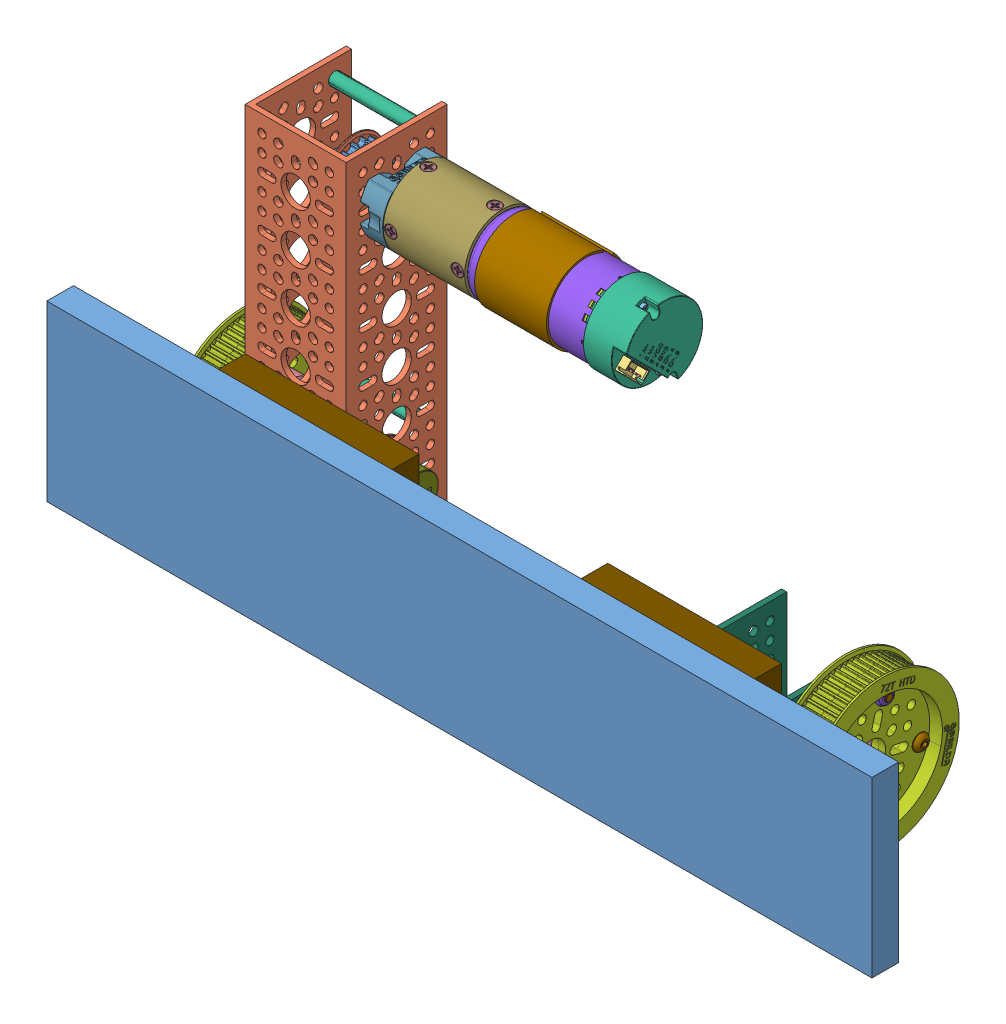
SolidWorks assembly moteurElevateur, configuration Défaut. Lengths in mm.
Overall size (392.22 189.33 92.57).
110 component instances, 36 part files, 9 mates.
Components (placement in the parent):
- plaqueMoteurElevateur-1: plaqueMoteurElevateur [Défaut] at (-14.6749 -16.481 385.8661) size (392.22 82.55 12.7)
- motorisationElevateur-1: motorisationElevateur [Défaut] at (-114.4008 36.5548 517.1661) x (0 -1 0) z (0 0 -1) size (189.33 304.42 86.33)
  - 1120-0006-0168 channel-1: 1120-0006-0168 channel [Défaut] at (77.0358 3.4821 146.5) x (0 -1 0) z (0 0 -1) size (48 168 48)
  - 5202-2402-0051 moteur-1: 5202-2402-0051 moteur [Défaut] at (-78.0426 -130.9533 205.1707) x (0 0 1) z (-1 0 0) size (52.36 150.75 52.36)
    - 5202-2402-0051.step-1: 5202-2402-0051.step [Défaut] at origin size (52.36 150.75 52.36)
      - 5000-0002-0001.step-1: 5000-0002-0001.step [Défaut] at origin size (52.36 88.75 52.36)
        - 5000-0002-0001 encoder cap.step-1: 5000-0002-0001 encoder cap.step [Défaut] x (0 1 0) z (0 0 1) size (22.84 52.33 52.33)
          - JST-XH-4POS-VERT (1).step-1: JST-XH-4POS-VERT (1).step [Défaut] at (2.8 12.25 -75.95) x (1 0 0) z (0 0 -1) size (10.4 12.83 12.83)
            - Plastic (1).step-1: Plastic (1).step [Défaut] at (-6.1146 -33.6358 -52.1967) x (0 0.707107 0.707107) z (-1 0 0) size (12.4 5.75 7)
            - Pin (1).step-1: Pin (1).step [Défaut] at (-7.7146 -29.3225 -51.2067) x (0 0.707107 0.707107) z (-1 0 0) size (0.64 0.64 10)
            - Pin (1).step-2: Pin (1).step [Défaut] at (-7.7146 -34.6258 -56.51) x (0 0.707107 0.707107) z (-1 0 0) size (0.64 0.64 10)
            - Pin (1).step-3: Pin (1).step [Défaut] at (-7.7146 -32.858 -54.7423) x (0 0.707107 0.707107) z (-1 0 0) size (0.64 0.64 10)
            - Pin (1).step-4: Pin (1).step [Défaut] at (-7.7146 -31.0902 -52.9745) x (0 0.707107 0.707107) z (-1 0 0) size (0.64 0.64 10)
          - screw.step-1: screw.step [Défaut] at (-41.264 -8.1646 3.9905) x (0.882398 0 0.470504) z (0 -1 0) size (8.86 7.85 4.95)
            - 99461A915_Phillips Rounded Head Thread-Forming Screws (1).step-1: 99461A915_Phillips Rounded Head Thread-Forming Screws (1).step [Défaut] at (27.264 -14.6475 -49.347) x (-0.332697 -0.623949 0.707107) z (-0.882398 0.470504 0) size (3.5 3.5 7.4)
          - screw_1.step-1: screw_1.step [Défaut] at (-14.4172 7.3354 3.9905) x (0.882398 0 0.470504) z (0 -1 0) size (8.86 7.85 4.95)
            - 99461A915_Phillips Rounded Head Thread-Forming Screws (1).step-1: 99461A915_Phillips Rounded Head Thread-Forming Screws (1).step [Défaut] at (-10.5142 -28.4382 -25.8237) x (-0.332697 -0.623949 0.707107) z (-0.882398 0.470504 0) size (3.5 3.5 7.4)
          - endcap.step-1: endcap.step [Défaut] at (72.6354 37.1707 -11.0784) x (0 -0.707107 -0.707107) z (1 0 0) size (37 37 21.84)
          - base.step-1: base.step [Défaut] at (-55.8646 37.1707 -11.0784) x (0 -0.707107 -0.707107) z (-1 0 0) size (34.96 34.31 1)
        - 5000-0002-0001 body.step-1: 5000-0002-0001 body.step [Défaut] at (-37.1707 3.4854 -11.0784) size (35.61 61.8 35.61)
        - 5000-0002-0001 motor shield.step-1: 5000-0002-0001 motor shield.step [Défaut] at (-37.1707 54.6354 -11.0784) x (0.808104 0 -0.58904) z (0 -1 0) size (37.5 37.27 34.15)
        - 5000-0002-0001 motor shaft.step-1: 5000-0002-0001 motor shaft.step [Défaut] at (-37.1707 59.4854 -11.0784) size (3.14 12.45 3.14)
      - 5102-0024-0051.step-1: 5102-0024-0051.step [Défaut] at origin size (36 76.68 35.98)
        - 5102 Gearbox Base.step-1: 5102 Gearbox Base.step [Défaut] at (-37.1707 60.1354 -11.0784) size (31.91 5.69 31.91)
        - 5102 Gearbox Barrel (3 stage, simple)_Gear Blank.step-1: 5102 Gearbox Barrel (3 stage, simple)_Gear Blank.step [Défaut] at (-37.1707 111.8354 -11.0784) x (1 0 0) z (0 -1 0) size (35.98 35.98 38.7)
        - 5102 Gearbox Barrel Screw (M3 x 8mm length Flat Head)_92010A118.step-1: 5102 Gearbox Barrel Screw (M3 x 8mm length Flat Head)_92010A118.step [Défaut] at (-37.1707 63.6354 5.0046) x (0.002439 -0.999997 0) z (0 0 1) size (5.46 5.46 8)
        - 5102 Gearbox Face.step-1: 5102 Gearbox Face.step [Défaut] at (-37.1707 93.3354 -11.0784) size (36 17.1 31.91)
        - 5102 Gearbox Bearing.step-1: 5102 Gearbox Bearing.step [Défaut] at (-37.1707 101.4354 -11.0784) size (17 5 17)
        - 5102 Gearbox Shaft (23.5mm Length, Simple).step-1: 5102 Gearbox Shaft (23.5mm Length, Simple).step [Défaut] at (-37.1707 89.9754 -11.0784) x (0.894773 0 -0.44652) z (0.44652 0 0.894773) size (8.97 40.6 8.97)
        - 5102 Gearbox Snap Ring.step-1: 5102 Gearbox Snap Ring.step [Défaut] at (-37.1707 106.5104 -11.0784) x (0 1 0) z (0 0 1) size (0.85 13.06 10.66)
        - 5102 Gearbox Barrel Screw (M3 x 8mm length Flat Head)_92010A118.step-2: 5102 Gearbox Barrel Screw (M3 x 8mm length Flat Head)_92010A118.step [Défaut] at (-37.1707 95.3354 5.0046) x (-0.002439 -0.999997 0) z (0 0 1) size (5.46 5.46 8)
        - 5102 Gearbox Barrel Screw (M3 x 8mm length Flat Head)_92010A118.step-3: 5102 Gearbox Barrel Screw (M3 x 8mm length Flat Head)_92010A118.step [Défaut] at (-21.0877 63.6354 -11.0784) x (0 -0.999997 -0.002439) z (1 0 0) size (5.46 5.46 8)
        - 5102 Gearbox Barrel Screw (M3 x 8mm length Flat Head)_92010A118.step-4: 5102 Gearbox Barrel Screw (M3 x 8mm length Flat Head)_92010A118.step [Défaut] at (-37.1707 63.6354 -27.1614) x (-0.002439 -0.999997 0) z (0 0 -1) size (5.46 5.46 8)
        - 5102 Gearbox Barrel Screw (M3 x 8mm length Flat Head)_92010A118.step-5: 5102 Gearbox Barrel Screw (M3 x 8mm length Flat Head)_92010A118.step [Défaut] at (-53.2537 63.6354 -11.0784) x (0 -0.999997 0.002439) z (-1 0 0) size (5.46 5.46 8)
        - 5102 Gearbox Barrel Screw (M3 x 8mm length Flat Head)_92010A118.step-6: 5102 Gearbox Barrel Screw (M3 x 8mm length Flat Head)_92010A118.step [Défaut] at (-21.0877 95.3354 -11.0784) x (0 -0.999997 0.002439) z (1 0 0) size (5.46 5.46 8)
        - 5102 Gearbox Barrel Screw (M3 x 8mm length Flat Head)_92010A118.step-7: 5102 Gearbox Barrel Screw (M3 x 8mm length Flat Head)_92010A118.step [Défaut] at (-37.1707 95.3354 -27.1614) x (0.002439 -0.999997 0) z (0 0 -1) size (5.46 5.46 8)
        - 5102 Gearbox Barrel Screw (M3 x 8mm length Flat Head)_92010A118.step-8: 5102 Gearbox Barrel Screw (M3 x 8mm length Flat Head)_92010A118.step [Défaut] at (-53.2537 95.3354 -11.0784) x (0 -0.999997 -0.002439) z (-1 0 0) size (5.46 5.46 8)
        - 5102 Gearbox Bearing.step-2: 5102 Gearbox Bearing.step [Défaut] at (-37.1707 93.3354 -11.0784) size (17 5 17)
        - 5102 Gearbox Base Mounting Screw M3 x 5mm length SHCS)_91290A110.step-1: 5102 Gearbox Base Mounting Screw M3 x 5mm length SHCS)_91290A110.step [Défaut] at (-46.0096 57.2554 -2.2396) x (0.056382 0 0.998409) z (0 -1 0) size (5.5 5.5 8)
        - 5102 Gearbox Base Mounting Screw M3 x 5mm length SHCS)_91290A110.step-2: 5102 Gearbox Base Mounting Screw M3 x 5mm length SHCS)_91290A110.step [Défaut] at (-28.3319 57.2554 -2.2396) x (0.998409 0 -0.056382) z (0 -1 0) size (5.5 5.5 8)
        - 5102 Gearbox Base Mounting Screw M3 x 5mm length SHCS)_91290A110.step-3: 5102 Gearbox Base Mounting Screw M3 x 5mm length SHCS)_91290A110.step [Défaut] at (-28.3319 57.2554 -19.9173) x (-0.056382 0 -0.998409) z (0 -1 0) size (5.5 5.5 8)
        - 5102 Gearbox Base Mounting Screw M3 x 5mm length SHCS)_91290A110.step-4: 5102 Gearbox Base Mounting Screw M3 x 5mm length SHCS)_91290A110.step [Défaut] at (-46.0096 57.2554 -19.9173) x (-0.998409 0 0.056382) z (0 -1 0) size (5.5 5.5 8)
  - 3417-1006-0016 assembly pulley-1: 3417-1006-0016 assembly pulley [Défaut] at (-89.9677 49.45 158.6429) x (0 1 0) z (1 0 0) size (12.01 27.98 27.98)
    - 3417-1006-0016 assembly.STEP-1: 3417-1006-0016 assembly.STEP [Défaut] at origin size (12.01 27.98 27.98)
      - 3417-1006-0016 body.STEP-1: 3417-1006-0016 body.STEP [Défaut] at (-62.7232 -4.1348 4.7756) size (12 23.97 23.97)
      - 3417-1006-0016 ring.STEP-1: 3417-1006-0016 ring.STEP [Défaut] at (-50.8429 9.3571 23.0035) x (0 -1 0) z (0 0 1) size (27.98 1.38 27.98)
      - 3417-1006-0016 ring.STEP-2: 3417-1006-0016 ring.STEP [Défaut] at (-60.0929 9.3571 23.0035) x (0 -1 0) z (0 0 -1) size (27.98 1.38 27.98)
      - 2806-0005-0006_91390A118.STEP-1: 2806-0005-0006_91390A118.STEP [Défaut] at (-55.4679 9.3571 17.1119) x (-0.607877 0.794031 0) z (0 0 -1) size (5.01 5.01 6.01)
  - 3417-1006-0016 assembly pulley-2: 3417-1006-0016 assembly pulley [Défaut] at (56.9629 49.45 143.4787) x (0 1 0) z (0.225568 0 0.974227) size (12.01 27.98 27.98)
    - 3417-1006-0016 assembly.STEP-1: 3417-1006-0016 assembly.STEP [Défaut] at origin size (12.01 27.98 27.98)
      - 3417-1006-0016 body.STEP-1: 3417-1006-0016 body.STEP [Défaut] at (-62.7232 -4.1348 4.7756) size (12 23.97 23.97)
      - 3417-1006-0016 ring.STEP-1: 3417-1006-0016 ring.STEP [Défaut] at (-50.8429 9.3571 23.0035) x (0 -1 0) z (0 0 1) size (27.98 1.38 27.98)
      - 3417-1006-0016 ring.STEP-2: 3417-1006-0016 ring.STEP [Défaut] at (-60.0929 9.3571 23.0035) x (0 -1 0) z (0 0 -1) size (27.98 1.38 27.98)
      - 2806-0005-0006_91390A118.STEP-1: 2806-0005-0006_91390A118.STEP [Défaut] at (-55.4679 9.3571 17.1119) x (-0.607877 0.794031 0) z (0 0 -1) size (5.01 5.01 6.01)
  - 1309-0016-1006 assembly-1: 1309-0016-1006 assembly [Défaut] at (37.2879 44.7557 158.8543) x (-0.848383 0 -0.529382) z (0 -1 0) size (28.36 32 10.95)
    - 1309-0016-1006 assembly.STEP-1: 1309-0016-1006 assembly.STEP [Défaut] at origin size (28.36 32 10.95)
      - 1309-0016-1006.STEP-1: 1309-0016-1006.STEP [Défaut] at (-18.2019 0.5776 8.7736) size (25.38 32 10)
      - 2800-0004-0014_90128A207.STEP-1: 2800-0004-0014_90128A207.STEP [Défaut] at (-16.149 11.6963 8.7736) x (0.5 -0.5 -0.707107) z (0.707107 0.707107 0) size (7 7 18.01)
      - 2800-0004-0014_90128A207.STEP-2: 2800-0004-0014_90128A207.STEP [Défaut] at (-20.2547 -10.5411 8.7736) x (-0.5 0.5 -0.707107) z (-0.707107 -0.707107 0) size (7 7 18.01)
  - 1501-0006-0430 renfort-1: 1501-0006-0430 renfort [Défaut] at (69.0358 3.4821 184) size (5.95 43.01 5.95)
  - 1501-0006-0430 renfort-2: 1501-0006-0430 renfort [Défaut] at (37.0358 3.4821 184) size (5.95 43.01 5.95)
  - 1501-0006-0430 renfort-3: 1501-0006-0430 renfort [Défaut] at (-82.9642 3.4821 184) size (5.95 43.01 5.95)
  - 1501-0006-0430 renfort-4: 1501-0006-0430 renfort [Défaut] at (-50.9642 3.4821 184) size (5.95 43.01 5.95)
  - 3402-0014-0072 pulley-1: 3402-0014-0072 pulley [Défaut] at (-4.0352 74.1976 188.4845) x (-0.974227 0 0.225568) z (0 -1 0) size (71.96 71.96 18.5)
    - 3402-0014-0072 assembly.STEP-1: 3402-0014-0072 assembly.STEP [Défaut] at origin size (71.96 71.96 18.5)
      - 3402-0014-0072.STEP-1: 3402-0014-0072.STEP [Défaut] at (-60.2208 7.0832 38.7155) size (71.96 71.96 10.5)
      - 3402-0014-0072.STEP-2: 3402-0014-0072.STEP [Défaut] at (-60.2208 7.0832 23.2155) x (0 -1 0) z (0 0 -1) size (71.96 71.96 10.5)
      - 2812-0004-0007_90576A103.STEP-1: 2812-0004-0007_90576A103.STEP [Défaut] at (-60.2208 31.0832 29.7155) x (0.866025 0.5 0) z (-0.5 0.866025 0) size (7.02 4.86 8.1)
      - 2812-0004-0007_90576A103.STEP-2: 2812-0004-0007_90576A103.STEP [Défaut] at (-60.2208 -16.9168 29.7155) x (0 1 0) z (-1 0 0) size (7.02 4.86 8.1)
      - 2812-0004-0007_90576A103.STEP-3: 2812-0004-0007_90576A103.STEP [Défaut] at (-84.2208 7.0832 32.2155) x (0.5 0.866025 0) z (0.866025 -0.5 0) size (7.02 4.86 8.1)
      - 2812-0004-0007_90576A103.STEP-4: 2812-0004-0007_90576A103.STEP [Défaut] at (-36.2208 7.0832 32.2155) x (1 0 0) z (0 -1 0) size (7.02 4.86 8.1)
      - 2802-0004-0010_92095A480.STEP-1: 2802-0004-0010_92095A480.STEP [Défaut] at (-36.2208 7.0832 25.5155) x (-0.923728 -0.383049 0) z (0 0 -1) size (13.53 12.99 15.57)
      - 2802-0004-0010_92095A480.STEP-2: 2802-0004-0010_92095A480.STEP [Défaut] at (-84.2208 7.0832 25.5155) x (0.923728 0.383049 0) z (0 0 -1) size (13.53 12.99 15.57)
      - 2802-0004-0010_92095A480.STEP-3: 2802-0004-0010_92095A480.STEP [Défaut] at (-60.2208 31.0832 36.4155) size (13.53 12.99 15.57)
      - 2802-0004-0010_92095A480.STEP-4: 2802-0004-0010_92095A480.STEP [Défaut] at (-60.2208 -16.9168 36.4155) x (-1 0 0) z (0 0 1) size (13.53 12.99 15.57)
  - 2801-0004-0008-rondelle-1: 2801-0004-0008-rondelle [Défaut] at (53.0358 29.9821 168) x (0.947224 0 -0.320572) z (0 -1 0) size (8 8 1)
  - 1611-0514-0006 Roulement-2: 1611-0514-0006 Roulement [Défaut] at (53.0358 28.9821 168) x (0.985961 0 0.166976) z (0.166976 0 -0.985961) size (15 5 15)
  - 2101-0006-0300-1: 2101-0006-0300 [Défaut] at (53.0358 -249.726 168) x (0.974227 0 -0.225568) z (0.225568 0 0.974227) size (6 300 5.5)
  - 1309-0016-1006 assembly-2: 1309-0016-1006 assembly [Défaut] at (63.1616 -244.2077 152.8636) x (0.529382 0 -0.848383) z (0 1 0) size (28.36 32 10.95)
    - 1309-0016-1006 assembly.STEP-1: 1309-0016-1006 assembly.STEP [Défaut] at origin size (28.36 32 10.95)
      - 1309-0016-1006.STEP-1: 1309-0016-1006.STEP [Défaut] at (-18.2019 0.5776 8.7736) size (25.38 32 10)
      - 2800-0004-0014_90128A207.STEP-1: 2800-0004-0014_90128A207.STEP [Défaut] at (-16.149 11.6963 8.7736) x (0.5 -0.5 -0.707107) z (0.707107 0.707107 0) size (7 7 18.01)
      - 2800-0004-0014_90128A207.STEP-2: 2800-0004-0014_90128A207.STEP [Défaut] at (-20.2547 -10.5411 8.7736) x (-0.5 0.5 -0.707107) z (-0.707107 -0.707107 0) size (7 7 18.01)
  - 2807-0609-1000-1: 2807-0609-1000 [Défaut] at (53.0358 -229.434 168) size (9 1 9)
  - 1611-0514-0006-3: 1611-0514-0006 [Défaut] at (53.0358 -223.434 168) x (-0.972788 0 0.231697) z (0.231697 0 0.972788) size (15 5 15)
  - 1120-0001-0048 u1-1: 1120-0001-0048 u1 [Défaut] at (77.0358 -203.434 146.5) x (0 -1 0) z (0 0 -1) size (48 48 48)
  - 1611-0514-0006-4: 1611-0514-0006 [Défaut] at (53.0358 -183.434 168) x (0.99995 0 -0.010033) z (0.010033 0 0.99995) size (15 5 15)
  - 2910-0919-0006 assembly collet-4: 2910-0919-0006 assembly collet [Défaut] at (21.0508 -173.9545 153.1256) x (-0.998275 0 0.058717) z (0.058717 0 0.998275) size (19 9.89 19.83)
    - 2910-0919-0006 assembly.STEP-1: 2910-0919-0006 assembly.STEP [Défaut] at origin size (19 9.89 19.83)
      - 2910-0919-0006.STEP-1: 2910-0919-0006.STEP [Défaut] at (-31.0565 -0.5204 16.7268) size (19 9.5 18.97)
      - 2800-0004-0010_90128A207.STEP-1: 2800-0004-0010_90128A207.STEP [Défaut] at (-24.2865 -0.5204 11.2868) x (0 -0.807243 -0.59022) z (1 0 0) size (7 7 14.01)
  - 3402-0014-0072 pulley-2: 3402-0014-0072 pulley [Défaut] at (-4.0352 -211.7186 188.4845) x (-0.974227 0 0.225568) z (0 -1 0) size (71.96 71.96 18.5)
    - 3402-0014-0072 assembly.STEP-1: 3402-0014-0072 assembly.STEP [Défaut] at origin size (71.96 71.96 18.5)
      - 3402-0014-0072.STEP-1: 3402-0014-0072.STEP [Défaut] at (-60.2208 7.0832 38.7155) size (71.96 71.96 10.5)
      - 3402-0014-0072.STEP-2: 3402-0014-0072.STEP [Défaut] at (-60.2208 7.0832 23.2155) x (0 -1 0) z (0 0 -1) size (71.96 71.96 10.5)
      - 2812-0004-0007_90576A103.STEP-1: 2812-0004-0007_90576A103.STEP [Défaut] at (-60.2208 31.0832 29.7155) x (0.866025 0.5 0) z (-0.5 0.866025 0) size (7.02 4.86 8.1)
      - 2812-0004-0007_90576A103.STEP-2: 2812-0004-0007_90576A103.STEP [Défaut] at (-60.2208 -16.9168 29.7155) x (0 1 0) z (-1 0 0) size (7.02 4.86 8.1)
      - 2812-0004-0007_90576A103.STEP-3: 2812-0004-0007_90576A103.STEP [Défaut] at (-84.2208 7.0832 32.2155) x (0.5 0.866025 0) z (0.866025 -0.5 0) size (7.02 4.86 8.1)
      - 2812-0004-0007_90576A103.STEP-4: 2812-0004-0007_90576A103.STEP [Défaut] at (-36.2208 7.0832 32.2155) x (1 0 0) z (0 -1 0) size (7.02 4.86 8.1)
      - 2802-0004-0010_92095A480.STEP-1: 2802-0004-0010_92095A480.STEP [Défaut] at (-36.2208 7.0832 25.5155) x (-0.923728 -0.383049 0) z (0 0 -1) size (13.53 12.99 15.57)
      - 2802-0004-0010_92095A480.STEP-2: 2802-0004-0010_92095A480.STEP [Défaut] at (-84.2208 7.0832 25.5155) x (0.923728 0.383049 0) z (0 0 -1) size (13.53 12.99 15.57)
      - 2802-0004-0010_92095A480.STEP-3: 2802-0004-0010_92095A480.STEP [Défaut] at (-60.2208 31.0832 36.4155) size (13.53 12.99 15.57)
      - 2802-0004-0010_92095A480.STEP-4: 2802-0004-0010_92095A480.STEP [Défaut] at (-60.2208 -16.9168 36.4155) x (-1 0 0) z (0 0 1) size (13.53 12.99 15.57)
  - 1611-0514-0006 Roulement-3: 1611-0514-0006 Roulement [Défaut] at (53.0358 -16.5179 168) x (1 0 0) z (0 0 -1) size (15 5 15)
  - 2910-0919-0006 assembly collet-5: 2910-0919-0006 assembly collet [Défaut] at (84.0923 -25.9975 151.2732) size (19 9.89 19.83)
    - 2910-0919-0006 assembly.STEP-1: 2910-0919-0006 assembly.STEP [Défaut] at origin size (19 9.89 19.83)
      - 2910-0919-0006.STEP-1: 2910-0919-0006.STEP [Défaut] at (-31.0565 -0.5204 16.7268) size (19 9.5 18.97)
      - 2800-0004-0010_90128A207.STEP-1: 2800-0004-0010_90128A207.STEP [Défaut] at (-24.2865 -0.5204 11.2868) x (0 -0.807243 -0.59022) z (1 0 0) size (7 7 14.01)
- blocElevateur-1: blocElevateur [Défaut] at (-100.6079 -16.481 373.1661) size (82.55 82.55 12.7)
- blocElevateur-2: blocElevateur [Défaut] at (71.7582 -16.481 373.1661) size (82.55 82.55 12.7)
Mates (geometry in assembly coordinates):
- Coïncidente2: coincident: plane of plaqueMoteurElevateur-1 through (-210.7829 24.794 398.5661) normal (0 1 0); plane of blocElevateur-1 through (-141.8829 24.794 385.8661) normal (0 1 0)
- Coïncidente3: coincident: plane of plaqueMoteurElevateur-1 through (-14.6749 -16.481 385.8661) normal (0 0 -1); plane of blocElevateur-1 through (-100.6079 -16.481 385.8661) normal (0 0 1)
- Coïncidente4: coincident: plane of motorisationElevateur-1/1120-0006-0168 channel-1 through (-141.8829 144.794 325.1661) normal (-1 0 0); plane of blocElevateur-1 through (-141.8829 24.794 385.8661) normal (-1 0 0)
- Coïncidente5: coincident: plane of motorisationElevateur-1/1120-0006-0168 channel-1 through (-93.8829 144.794 373.1661) normal (0 0 1); plane of blocElevateur-1 through (-100.6079 -16.481 373.1661) normal (0 0 -1)
- Distance2: distance = 46.1081 mm: plane of motorisationElevateur-1/2101-0006-0300-1 through (-164.6749 -16.481 349.1661) normal (-1 0 0); plane of plaqueMoteurElevateur-1 through (-210.7829 24.794 398.5661) normal (-1 0 0)
- Coïncidente10: coincident: plane of plaqueMoteurElevateur-1 through (-210.7829 -57.756 398.5661) normal (0 -1 0); plane of blocElevateur-2 through (30.4832 -57.756 385.8661) normal (0 -1 0)
- Coïncidente11: coincident: plane of plaqueMoteurElevateur-1 through (-14.6749 -16.481 385.8661) normal (0 0 -1); plane of blocElevateur-2 through (71.7582 -16.481 385.8661) normal (0 0 1)
- Coïncidente12: coincident: plane of motorisationElevateur-1/1120-0001-0048 u1-1 through (113.0332 24.794 325.1661) normal (1 0 0); plane of blocElevateur-2 through (113.0332 24.794 385.8661) normal (1 0 0)
- Distance3: distance = 17.275 mm: plane of motorisationElevateur-1/1120-0001-0048 u1-1 through (89.0332 7.519 370.6661) normal (0 1 0); plane of blocElevateur-2 through (30.4832 24.794 385.8661) normal (0 1 0)
